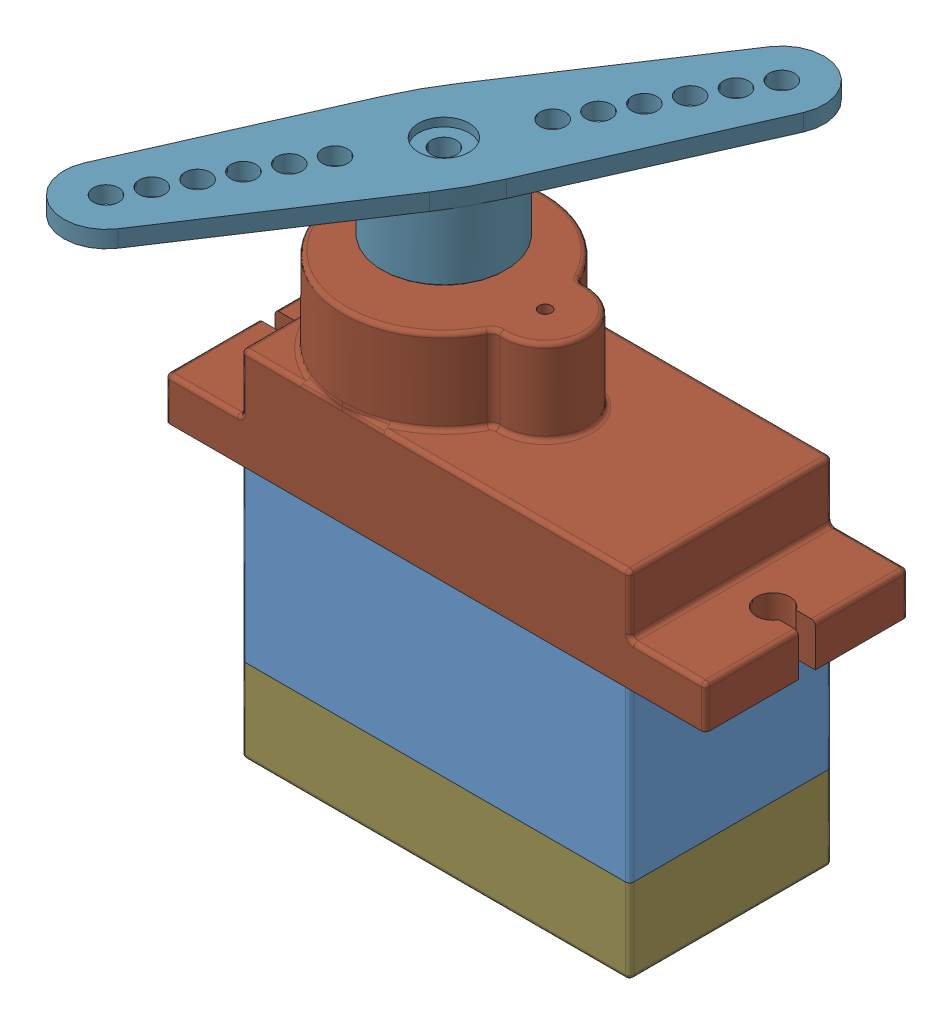
SolidWorks assembly SERVO, configuration Default. Lengths in mm.
Overall size (33 31.96 33.81).
26 component instances, 15 part files, 50 mates.
Components (placement in the parent):
- middle cover-1: middle cover [Default] at (8.87 8.8972 15.8774) size (23 11 12)
- shaft-1: shaft [Default] at (3.37 15.3972 15.8774) x (0 1 0) z (0.930169 0 0.367132) size (14.5 8.25 8.81)
- part 1-1: part 1 [Default] at (3.37 15.7972 15.8774) x (0 0 1) z (1 0 0) size (9.5 5.14 9.55)
- gear_sub1-1: gear_sub1 [Default] at (9.5 19.3472 15.8774) x (0.314237 0 0.949345) z (-0.949345 0 0.314237) size (10.24 10.65 10.25)
  - shaft^gear_sub1-1: shaft^gear_sub1 [Default] at origin size (1 10.65 1) (virtual)
  - spur gear_iso-2: spur gear_iso [ISO - Spur gear 0.25M 39T 20PA 1FW ---S39A75H50L0.8N] at (0 0.1 0) x (0 1 0) z (0 0 1) size (1 10.24 10.25)
  - spur gear_iso-5: spur gear_iso [ISO - Spur gear 0.25M 10T 20PA 1.75FW ---S10A75H50L1.0N] at (0 1.1 0) x (0 1 0) z (0 0 1) size (1.75 2.87 3)
- gear_sub2-1: gear_sub2 [Default] at (3.37 20.7972 15.8774) x (0.27641 0 0.96104) z (-0.96104 0 0.27641) size (10.24 2.75 10.25)
  - spur gear_iso-2: spur gear_iso [ISO - Spur gear 0.25M 39T 20PA 1FW ---S39A75H50L0.8N] at (0 0.1 0) x (0 1 0) z (0 0 1) size (1 10.24 10.25)
  - spur gear_iso-5: spur gear_iso [ISO - Spur gear 0.25M 10T 20PA 1.75FW ---S10A75H50L1.0N] at (0 1.1 0) x (0 1 0) z (0 0 1) size (1.75 2.87 3)
- pcb-1: pcb [Default] at (4.7516 11.69 15.8774) x (0.906308 0.422618 0) z (0 0 -1) size (10 2 9)
- wires1^SERVO-1: wires1^SERVO [Default] at (8.87 8.8972 21.8774) (virtual)
- DC Motor as part-2: DC Motor as part [Default] at (20.0465 3.7393 19.3612) x (0 0 -1) z (0 1 0) size (8.04 6.55 11.14)
- Rotor scaled-1: Rotor scaled [Default] at (15.62 14.0372 15.8774) x (0.525194 0 -0.850983) z (0 1 0) size (5.2 7.1 15.2)
- spur gear_am-3: spur gear_am [Metric - Spur gear 0.25M 10T 20PA 2FW ---S10N75H50L0.8N] at (15.62 18.9472 15.8774) x (0 1 0) z (0.468546 0 0.883439) size (2 2.87 3)
- gear_sub3-2: gear_sub3 [Default] at (7.9761 21.8914 15.1354) x (-0.999976 0 0.00696) z (-0.00696 0 -0.999976) size (10.24 7 10.25)
  - spur gear_iso-2: spur gear_iso [ISO - Spur gear 0.25M 39T 20PA 1FW ---S39A75H50L0.8N] at (-1.5188 0.3058 -0.7526) x (0 1 0) z (0 0 1) size (1 10.24 10.25)
  - spur gear_iso-6: spur gear_iso [ISO - Spur gear 0.25M 10T 20PA 6FW ---S10A75H50L0.8N] at (-1.5188 1.3058 -0.7526) x (0 1 0) z (0 0 1) size (6 2.87 3)
- gear5-1: gear5 [Default] at (6.2114 -19.0533 16.4017) x (0 -1 0) z (-0.719067 0 -0.694941) size (6.5 10.24 10.25)
- Part5-1: Part5 [Default] at (8.87 24.8972 15.8774) size (32 11 12.1)
- part 3 bottom-1: part 3 bottom [Default] at (8.87 3.8972 15.8774) size (23 5 12)
- Part6-1: Part6 [Default] at (-1.38 3.7472 11.1274) x (0 1 0) z (-0.44899 0 0.893537) size (20.01 2 2)
- Part6-2: Part6 [Default] at (-1.38 3.7472 20.6274) x (0 1 0) z (-0.272553 0 0.962141) size (20.01 2 2)
- Part6-4: Part6 [Default] at (19.12 3.7472 20.6274) x (0 1 0) z (-0.058733 0 0.998274) size (20.01 2 2)
- Part6-6: Part6 [Default] at (19.12 3.7472 11.1274) x (0 1 0) z (0.17693 0 0.984223) size (20.01 2 2)
- Part7-1: Part7 [Default] at (3.37 35.6972 15.8774) x (0.877667 0 0.47927) z (0.47927 0 -0.877667) size (7.36 5 34.5)
Mates (geometry in assembly coordinates):
- Concentric1: concentric anti-aligned: cylinder of middle cover-1 through (3.37 8.8962 15.8774) axis (0 1 0) radius 5; cylinder of part 1-1 through (3.37 16.2972 15.8774) axis (0 -1 0) radius 4.75
- Concentric2: concentric aligned: cylinder of shaft-1 through (3.37 15.3972 15.8774) axis (0 -1 0) radius 0.6; cylinder of part 1-1 through (3.37 19.2972 15.8774) axis (0 -1 0) radius 4.5
- Tangent1: tangent: plane of assembly; face of shaft-1; plane of part 1-1 through (4.8064 16.4472 14.6722) normal (0 1 0)
- Concentric3: concentric aligned: cylinder of shaft-1 through (3.37 15.3972 15.8774) axis (0 -1 0) radius 0.5; cylinder of gear_sub2-1/spur gear_iso-5 through (3.37 71.8973 15.8774) axis (0 -1 0) radius 0.5
- Coincident6: coincident anti-aligned: plane of shaft-1 through (3.1865 20.8972 16.3425) normal (0 1 0); plane of gear_sub2-1/spur gear_iso-2 through (3.37 20.8972 15.8774) normal (0 -1 0)
- Concentric4: concentric aligned: cylinder of middle cover-1 through (9.5 19.4472 15.8774) axis (0 -1 0) radius 0.5; cylinder of gear_sub1-1/shaft^gear_sub1-1 through (9.5 18.6972 15.8774) axis (0 -1 0) radius 0.5
- Width1: width anti-aligned: plane of pcb-1 through (9.6001 13.1234 20.3774) normal (0 0 1); plane of pcb-1 through (9.6001 13.1234 11.3774) normal (0 0 -1); plane of middle cover-1 through (20.37 18.8972 20.8774) normal (0 0 -1); plane of middle cover-1 through (20.37 18.8972 10.8774) normal (0 0 1)
- Coincident9: coincident: plane of middle cover-1 through (8.87 8.8972 15.8774) normal (0 -1 0); line of pcb-1 through (0.537 8.8972 20.3774) axis (0 0 -1)
- Angle1: planar angle = 0.436332 rad aligned: plane of pcb-1 through (5.0685 11.0103 15.8774) normal (0.422618 -0.906308 0); plane of middle cover-1 through (8.87 8.8972 15.8774) normal (0 -1 0)
- Tangent2: tangent: cylinder of middle cover-1 through (-1.38 18.8972 20.6274) axis (0 -1 0) radius 1.6; line of pcb-1 through (0.22 9.5769 20.3774) axis (0 0 -1)
- InPlace1: in place: plane of middle cover-1 through (20.37 18.8972 21.8774) normal (0 0 1); plane of ? through (0 0 21.8774) normal (0 0 1); moOrthogonalPlaneRef_w of middle cover-1 through (20.37 18.8972 21.8774) normal (0 0 1); plane of ? through (0 0 21.8774) normal (0 1 0); plane of middle cover-1 through (20.37 18.8972 21.8774) normal (0 0 1); plane of ? through (0 0 21.8774) normal (1 0 0); plane of middle cover-1 through (20.37 18.8972 21.8774) normal (0 0 1); unknown of wires1^SERVO-1
- Coincident11: coincident aligned: plane of middle cover-1; plane of wires1^SERVO-1
- Coincident12: coincident aligned: moOrthogonalPlaneRef_w of middle cover-1 through (8.87 8.8972 21.8774) normal (0 1 0); plane of wires1^SERVO-1 through (8.87 8.8972 21.8774) normal (0 1 0)
- Coincident13: coincident anti-aligned: moOrthogonalPlaneRef_w of middle cover-1 through (8.87 8.8972 21.8774) normal (-1 0 0); plane of wires1^SERVO-1 through (8.87 8.8972 21.8774) normal (1 0 0)
- Concentric5: concentric aligned: cylinder of middle cover-1 through (15.62 8.8962 15.8774) axis (0 1 0) radius 1.55; cylinder of DC Motor as part-2 through (15.62 17.7472 15.8774) axis (0 1 0) radius 0.4
- Parallel5: parallel anti-aligned: plane of middle cover-1 through (12.22 12.8972 19.2524) normal (1 0 0); plane of DC Motor as part-2 through (12.62 17.8972 18.5231) normal (-1 0 0)
- Coincident11: coincident anti-aligned: plane of middle cover-1 through (8.87 17.8972 15.8774) normal (0 -1 0); plane of DC Motor as part-2 through (15.62 17.8972 15.8774) normal (0 1 0)
- Coincident12: coincident anti-aligned: circle of DC Motor as part-2; cylinder of Rotor scaled-1 through (15.62 21.6372 15.8774) axis (0 -1 0) radius 0.4
- Coincident13: coincident aligned: plane of DC Motor as part-2 through (14.486 9.2572 14.5254) normal (0 -1 0); plane of Rotor scaled-1 through (15.62 9.2572 15.8774) normal (0 -1 0)
- Coincident15: coincident anti-aligned: plane of middle cover-1 through (8.87 15.2972 15.8774) normal (0 1 0); plane of part 1-1 through (3.37 15.2972 15.8774) normal (0 -1 0)
- Parallel7: parallel aligned: plane of middle cover-1 through (4.62 14.7972 10.8774) normal (1 0 0); plane of part 1-1 through (4.37 15.2972 15.8774) normal (1 0 0)
- Concentric7: concentric aligned: cylinder of Rotor scaled-1 through (15.62 21.6372 15.8774) axis (0 -1 0) radius 0.4; cylinder of spur gear_am-3 through (15.62 68.9473 15.8774) axis (0 -1 0) radius 0.4
- Width2: width aligned: plane of gear_sub1-1/spur gear_iso-2 through (9.5 20.4472 15.8774) normal (0 1 0); plane of spur gear_am-3 through (9.5 19.4472 15.8774) normal (0 -1 0); plane of gear_sub1-1/spur gear_iso-2 through (15.62 20.9472 15.8774) normal (0 1 0); plane of spur gear_am-3 through (15.62 18.9472 15.8774) normal (0 -1 0)
- Lock1: lock: unknown of Rotor scaled-1; unknown of spur gear_am-3
- Concentric8: concentric anti-aligned: cylinder of gear_sub1-1/shaft^gear_sub1-1 through (9.5 18.6972 15.8774) axis (0 1 0) radius 0.5; cylinder of gear_sub3-2/spur gear_iso-6 through (9.5 73.1973 15.8774) axis (0 -1 0) radius 0.4
- Coincident16: coincident anti-aligned: plane of gear_sub1-1/spur gear_iso-5 through (9.5 22.1972 15.8774) normal (0 1 0); plane of gear_sub3-2/spur gear_iso-2 through (9.5 22.1972 15.8774) normal (0 -1 0)
- Concentric9: concentric anti-aligned: cylinder of shaft-1 through (3.37 15.3972 15.8774) axis (0 -1 0) radius 0.6; cylinder of gear5-1 through (3.37 -20.8028 15.8774) axis (0 1 0) radius 0.5
- GearMate5: gear = 39 : 10 mm: cylinder of spur gear_am-3 through (15.62 20.9472 15.8774) axis (0 -1 0) radius 0.9365; cylinder of gear_sub1-1/spur gear_iso-2 through (9.5 20.4472 15.8774) axis (0 -1 0) radius 4.5615
- GearMate6: gear = 39 : 10 mm: cylinder of gear_sub1-1/spur gear_iso-5 through (9.5 22.1972 15.8774) axis (0 -1 0) radius 0.9365; cylinder of gear_sub2-1/spur gear_iso-2 through (3.37 21.8972 15.8774) axis (0 -1 0) radius 4.5615
- GearMate7: gear = 39 : 10 mm: cylinder of gear_sub2-1/spur gear_iso-5 through (3.37 23.6472 15.8774) axis (0 -1 0) radius 0.9365; cylinder of gear_sub3-2/spur gear_iso-2 through (9.5 23.1972 15.8774) axis (0 -1 0) radius 4.5615
- GearMate8: gear = 39 : 10 mm: cylinder of gear_sub3-2/spur gear_iso-6 through (9.5 29.1972 15.8774) axis (0 -1 0) radius 0.9365; cylinder of gear5-1 through (3.37 26.1972 15.8774) axis (0 1 0) radius 4.5615
- Coincident17: coincident aligned: plane of gear_sub3-2/spur gear_iso-6 through (9.5 29.1972 15.8774) normal (0 1 0); plane of gear5-1 through (3.37 29.1972 15.8774) normal (0 1 0)
- Lock3: lock: unknown of shaft-1; unknown of gear5-1
- Concentric11: concentric anti-aligned: cylinder of middle cover-1 through (-1.38 19.8972 20.6274) axis (0 -1 0) radius 1; cylinder of Part5-1 through (-1.38 18.8972 20.6274) axis (0 1 0) radius 1
- Concentric12: concentric anti-aligned: cylinder of middle cover-1 through (19.12 19.8972 11.1274) axis (0 -1 0) radius 1; cylinder of Part5-1 through (19.12 18.8972 11.1274) axis (0 1 0) radius 1
- Coincident18: coincident anti-aligned: plane of middle cover-1 through (8.87 18.8972 15.8774) normal (0 1 0); plane of Part5-1 through (8.87 18.8972 15.8774) normal (0 -1 0)
- Coincident19: coincident anti-aligned: plane of middle cover-1 through (8.87 8.8972 15.8774) normal (0 -1 0); plane of part 3 bottom-1 through (8.87 8.8972 15.8774) normal (0 1 0)
- Concentric13: concentric aligned: cylinder of middle cover-1 through (-1.38 18.8972 20.6274) axis (0 -1 0) radius 0.6; cylinder of part 3 bottom-1 through (-1.38 8.8972 20.6274) axis (0 -1 0) radius 1
- Concentric14: concentric aligned: cylinder of middle cover-1 through (19.12 18.8972 20.6274) axis (0 -1 0) radius 0.6; cylinder of part 3 bottom-1 through (19.12 8.8972 20.6274) axis (0 -1 0) radius 1
- Concentric16: concentric aligned: cylinder of part 3 bottom-1 through (-1.38 7.2472 11.1274) axis (0 -1 0) radius 0.6; cylinder of Part6-1 through (-1.38 3.7472 11.1274) axis (0 -1 0) radius 0.5
- Coincident22: coincident anti-aligned: plane of part 3 bottom-1 through (-1.38 4.7472 11.1274) normal (0 -1 0); plane of Part6-1 through (-1.8267 4.7472 10.9029) normal (0 1 0)
- Concentric17: concentric aligned: cylinder of part 3 bottom-1 through (-1.38 7.2472 20.6274) axis (0 -1 0) radius 0.6; cylinder of Part6-2 through (-1.38 3.7472 20.6274) axis (0 -1 0) radius 0.5
- Coincident23: coincident anti-aligned: plane of part 3 bottom-1 through (-1.38 4.7472 20.6274) normal (0 -1 0); plane of Part6-2 through (-1.861 4.7472 20.4911) normal (0 1 0)
- Concentric18: concentric aligned: cylinder of part 3 bottom-1 through (19.12 7.2472 20.6274) axis (0 -1 0) radius 0.6; cylinder of Part6-4 through (19.12 3.7472 20.6274) axis (0 -1 0) radius 0.5
- Coincident24: coincident anti-aligned: plane of part 3 bottom-1 through (19.12 4.7472 20.6274) normal (0 -1 0); plane of Part6-4 through (18.6209 4.7472 20.598) normal (0 1 0)
- Concentric19: concentric aligned: cylinder of part 3 bottom-1 through (19.12 7.2472 11.1274) axis (0 -1 0) radius 0.6; cylinder of Part6-6 through (19.12 3.7472 11.1274) axis (0 -1 0) radius 0.5
- Coincident25: coincident anti-aligned: plane of part 3 bottom-1 through (19.12 4.7472 11.1274) normal (0 -1 0); plane of Part6-6 through (18.6279 4.7472 11.2158) normal (0 1 0)
- Coincident26: coincident anti-aligned: plane of gear5-1 through (3.37 32.6972 15.8774) normal (0 1 0); plane of Part7-1 through (3.37 32.6972 15.8774) normal (0 -1 0)
- Concentric20: concentric aligned: cylinder of gear5-1 through (3.37 -20.8028 15.8774) axis (0 1 0) radius 0.5; cylinder of Part7-1 through (3.37 30.6972 15.8774) axis (0 1 0) radius 0.75
- Lock4: lock: unknown of gear5-1; unknown of Part7-1
